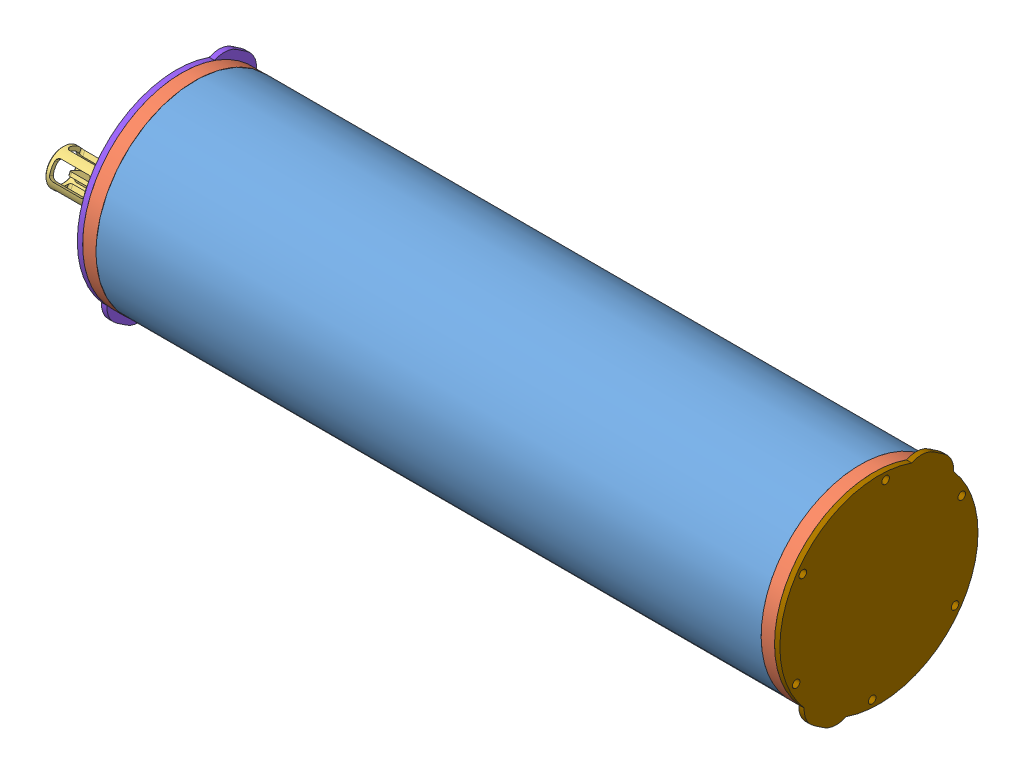
SolidWorks assembly BRPT_v2, configuration Default. Lengths in mm.
Overall size (357.59 209.76 319.54).
48 component instances, 19 part files, 0 mates.
Components (placement in the parent):
- BRPT_v1-1: BRPT_v1 [Default] at (360.8429 123.3491 426.7713) x (0 1 0) z (0 0 1) size (209.76 357.59 319.54)
  - 3in series housing-1: 3in series housing [Default] at (162.5946 57.9765 268.4972) size (88.9 298.45 88.9)
  - 3in series Oring flange-1: 3in series Oring flange [Default] at (162.5946 335.4265 268.4972) x (-0.99734 0 0.072895) z (0 -1 0) size (88.9 88.9 27.11)
  - 3in series Oring flange-2: 3in series Oring flange [Default] at (162.5946 78.9765 268.4972) x (0.99734 0 -0.072895) z (0 1 0) size (88.9 88.9 27.11)
  - CELSIUS-TEMPERATURE-SENSOR-ASSEMBLY-X1-1: CELSIUS-TEMPERATURE-SENSOR-ASSEMBLY-X1 [Default] at (122.5922 326.5947 279.9307) x (0.457003 0 0.889465) z (0 1 0) size (18 16 56.58)
  - BAR30-SENSOR-ASSEMBLY-R1-1: BAR30-SENSOR-ASSEMBLY-R1 [Default] at (177.0309 360.3608 268.6158) x (-0.789833 0 0.613322) z (0 1 0) size (18 16 37.53)
  - PENETRATOR-M-NUT-10-8-R2-1: PENETRATOR-M-NUT-10-8-R2 [Default] at (151.3587 362.4265 251.9517) x (0.587103 0 -0.809513) z (0 -1 0) size (18 16 9.22)
  - VENT-M-BOLT-10-25-A-R4-1: VENT-M-BOLT-10-25-A-R4 [94036A625] at (151.3587 363.5765 251.9517) x (0.845284 0 0.534318) z (0 1 0) size (18 16 39.53)
  - VENT-M-PLUG-10-A-R3-1: VENT-M-PLUG-10-A-R3 [Default] at (151.3587 367.5765 251.9517) x (-0.985482 0 -0.169779) z (0 -1 0) size (18 17.99 20.15)
  - PENETRATOR-M-NUT-10-8-R2-2: PENETRATOR-M-NUT-10-8-R2 [Default] at (180.598 354.4265 277.208) x (-0.220712 0 -0.975339) z (0 1 0) size (18 16 9.22)
  - PENETRATOR-M-NUT-10-8-R2-3: PENETRATOR-M-NUT-10-8-R2 [Default] at (164.0525 362.4265 288.444) x (-0.986467 0 -0.16396) z (0 -1 0) size (18 16 9.22)
  - 3in series end cap 3 holes-1: 3in series end cap 3 holes [Default] at (162.5946 362.4265 268.4972) x (-0.827274 0 0.561799) z (-0.561799 0 -0.827274) size (96 2.4 88.9)
  - 3in series end cap-2: 3in series end cap [Default] at (162.5946 49.5765 268.4972) x (-0.827274 0 0.561799) z (-0.561799 0 -0.827274) size (96 2.4 88.9)
  - Battery holder-1: Battery holder [Default] at (88.5633 90.8064 358.6088) x (-0.32029 0 -0.94732) z (0.94732 0 -0.32029) size (98.62 218.61 98.22)
    - battery holder v2-1: battery holder v2 [Default] at (61.653 68.5201 98.9932) size (71.12 137.5 69.24)
    - 2600mAh Battery-1: 2600mAh Battery [Default] at (86.0749 4.0582 84.8932) x (-0.71885 0 -0.695165) z (0.695165 0 -0.71885) size (18 65 18) (hidden)
    - 2600mAh Battery-2: 2600mAh Battery [Default] at (86.0749 134.0582 84.8932) x (0.792584 0 -0.609763) z (-0.609763 0 -0.792584) size (18 65 18) (hidden)
    - 2600mAh Battery-3: 2600mAh Battery [Default] at (37.231 4.0582 113.0932) size (18 65 18) (hidden)
    - 2600mAh Battery-4: 2600mAh Battery [Default] at (37.231 134.0582 113.0932) x (0.840955 0 0.541105) z (0.541105 0 -0.840955) size (18 65 18) (hidden)
    - 2600mAh Battery-5: 2600mAh Battery [Default] at (61.653 4.0582 127.1932) x (-0.28708 0 -0.957907) z (0.957907 0 -0.28708) size (18 65 18) (hidden)
    - 2600mAh Battery-6: 2600mAh Battery [Default] at (61.653 69.0582 127.1932) x (-0.79051 0 -0.612449) z (0.612449 0 -0.79051) size (18 65 18) (hidden)
    - 2600mAh Battery-7: 2600mAh Battery [Default] at (37.231 4.0582 84.8932) size (18 65 18) (hidden)
    - 2600mAh Battery-8: 2600mAh Battery [Default] at (37.231 69.0582 84.8932) x (-0.486699 0 -0.87357) z (0.87357 0 -0.486699) size (18 65 18) (hidden)
    - Battery holder endcap-1: Battery holder endcap [Default] at (99.0192 180.1854 40.1409) x (-1 0 0) z (0 0 1) size (75.69 15.3 75.69)
      - Battery holder endcap-1: Battery holder endcap [Default] at (37.3662 31.3154 58.8523) size (75.69 14.1 75.69)
      - battery contact 209-2: battery contact 209 [Default] at (9.8065 42.9154 70.2374) x (0 1 0) z (0.5 0 0.866025) size (6.42 12.29 7.92)
      - battery contact 209-3: battery contact 209 [Default] at (33.4462 42.9154 88.4123) x (0 1 0) z (1 0 0) size (6.42 12.29 7.92)
      - battery contact 209-4: battery contact 209 [Default] at (61.0059 42.9154 77.0271) x (0 1 0) z (0.5 0 -0.866025) size (6.42 12.29 7.92)
      - battery contact 209-5: battery contact 209 [Default] at (64.9259 42.9154 47.4671) x (0 1 0) z (-0.5 0 -0.866025) size (6.42 12.29 7.92)
      - battery contact 209-6: battery contact 209 [Default] at (41.2862 42.9154 29.2923) x (0 1 0) z (-1 0 0) size (6.42 12.29 7.92)
      - battery contact 209-7: battery contact 209 [Default] at (13.7265 42.9154 40.6774) x (0 1 0) z (-0.5 0 0.866025) size (6.42 12.29 7.92)
    - Battery holder endcap-2: Battery holder endcap [Default] at (24.2867 -43.1453 40.1409) size (75.69 15.3 75.69)
      - Battery holder endcap-1: Battery holder endcap [Default] at (37.3662 31.3154 58.8523) size (75.69 14.1 75.69)
      - battery contact 209-2: battery contact 209 [Default] at (9.8065 42.9154 70.2374) x (0 1 0) z (0.5 0 0.866025) size (6.42 12.29 7.92)
      - battery contact 209-3: battery contact 209 [Default] at (33.4462 42.9154 88.4123) x (0 1 0) z (1 0 0) size (6.42 12.29 7.92)
      - battery contact 209-4: battery contact 209 [Default] at (61.0059 42.9154 77.0271) x (0 1 0) z (0.5 0 -0.866025) size (6.42 12.29 7.92)
      - battery contact 209-5: battery contact 209 [Default] at (64.9259 42.9154 47.4671) x (0 1 0) z (-0.5 0 -0.866025) size (6.42 12.29 7.92)
      - battery contact 209-6: battery contact 209 [Default] at (41.2862 42.9154 29.2923) x (0 1 0) z (-1 0 0) size (6.42 12.29 7.92)
      - battery contact 209-7: battery contact 209 [Default] at (13.7265 42.9154 40.6774) x (0 1 0) z (-0.5 0 0.866025) size (6.42 12.29 7.92)
    - 92239A100_FLANGED WING NUT-1: 92239A100_FLANGED WING NUT [92239A100] at (61.653 -11.8299 98.9932) x (1 0 0) z (0 1 0) size (22.23 15.88 11.75)
    - 92239A100_FLANGED WING NUT-2: 92239A100_FLANGED WING NUT [92239A100] at (61.653 148.8701 98.9932) x (1 0 0) z (0 -1 0) size (22.23 15.88 11.75)
    - 91565A345_LOW-STRENGTH STEEL THREADED ROD-1: 91565A345_LOW-STRENGTH STEEL THREADED ROD [91565A345] at (61.653 69.9701 98.9932) x (0 1 0) z (-0.704559 0 -0.709645) size (179.29 4.22 4.81)
    - Battery holder spacer-1: Battery holder spacer [Default] at (61.653 -7.5935 98.9932) x (0.5 0 -0.866025) z (-0.866025 0 -0.5) size (71.12 9 73.26)
  - Electronics Shelf-2: Electronics Shelf [Default] at (184.5849 247.1362 219.3245) x (0.32029 0 0.94732) z (-0.94732 0 0.32029) size (74.93 81.28 51.4)
    - Electronics Shelf-1: Electronics Shelf [Default] at (39.539 0.3112 46.7413) size (74.93 81.28 33.74)
    - 93505A103_MALE-FEMALE THREADED HEX STANDOFF-2: 93505A103_MALE-FEMALE THREADED HEX STANDOFF [93505A103] at (64.5455 76.1098 32.9301) x (0 0 -1) z (1 0 0) size (17.78 5.5 4.76)
    - 93505A103_MALE-FEMALE THREADED HEX STANDOFF-3: 93505A103_MALE-FEMALE THREADED HEX STANDOFF [93505A103] at (14.5455 76.1098 32.9301) x (0 0 -1) z (1 0 0) size (17.78 5.5 4.76)
    - PCB-1: PCB [Default] at (39.5455 41.1098 28.9613) x (1 0 0) z (0 1 0) size (60 2.54 80)
